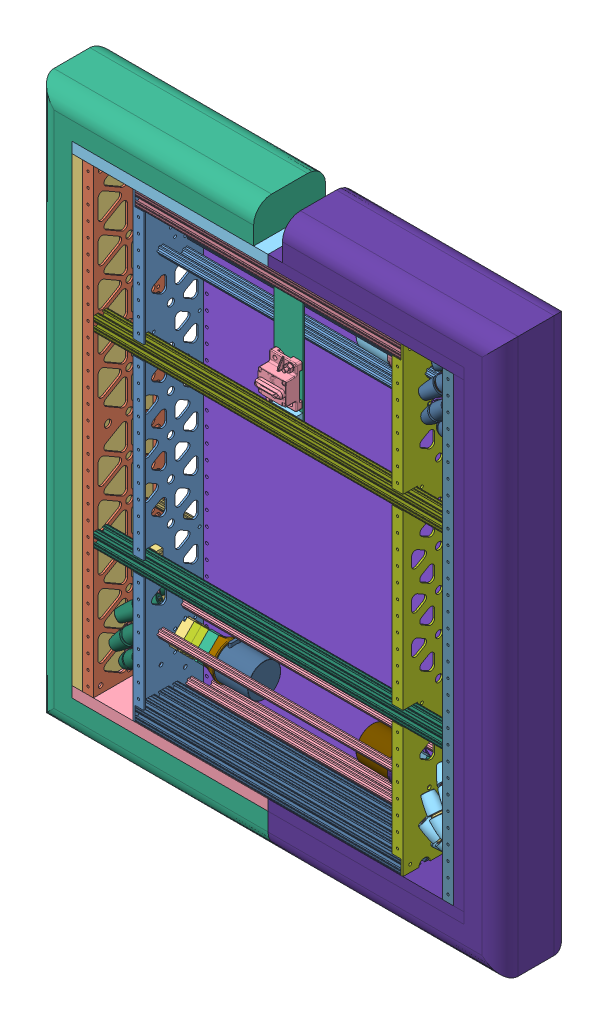
SolidWorks assembly Copy of Fame 2020, configuration Default. Lengths in mm. (continued)
Components (placement in the parent): (continued)
- Left Wheel Assembly v4(Mirror)^Copy of Fame 2020-1: Left Wheel Assembly v4(Mirror)^Copy of Fame 2020 [Default] at (-500 0 0) x (-1 0 0) z (0 0 -1) size (65.82 166.11 165.01) (virtual)
  - 6_Mecanum_Wheel_Left_217-2799 v1(Mirror)^Left Wheel Assembly v4(Mirror)_Copy of Fame 2020-1: 6_Mecanum_Wheel_Left_217-2799 v1(Mirror)^Left Wheel Assembly v4(Mirror)_Copy of Fame 2020 [Default] x (0 0 -1) z (1 0 0) size (165.01 166.11 65.82) (virtual)
    - 217-2799-001 Rev1(Mirror)^6_Mecanum_Wheel_Left_217-2799 v1(Mirror)_Left Wheel Assembly v4(Mirror)_Copy of Fame 2020-1: 217-2799-001 Rev1(Mirror)^6_Mecanum_Wheel_Left_217-2799 v1(Mirror)_Left Wheel Assembly v4(Mirror)_Copy of Fame 2020 [Default] at (33.3875 -317.5 -234.0098) x (0.707107 0.707107 0) z (0 0 1) size (95.78 100.46 28.55) (virtual)
    - 217-2799-001 Rev1(Mirror)^6_Mecanum_Wheel_Left_217-2799 v1(Mirror)_Left Wheel Assembly v4(Mirror)_Copy of Fame 2020-2: 217-2799-001 Rev1(Mirror)^6_Mecanum_Wheel_Left_217-2799 v1(Mirror)_Left Wheel Assembly v4(Mirror)_Copy of Fame 2020 [Default] at (33.3875 -317.5 -221.3098) x (-0.987688 -0.156434 0) z (0 0 -1) size (95.78 100.46 28.55) (virtual)
    - 217-2799-002 Rev1(Mirror)^6_Mecanum_Wheel_Left_217-2799 v1(Mirror)_Left Wheel Assembly v4(Mirror)_Copy of Fame 2020-1: 217-2799-002 Rev1(Mirror)^6_Mecanum_Wheel_Left_217-2799 v1(Mirror)_Left Wheel Assembly v4(Mirror)_Copy of Fame 2020 [Default] at (4.057 -346.8305 -227.6598) x (-0.707107 0.707107 0) z (0.707107 0.707107 0) size (26.84 25.39 30.1) (virtual)
    - 217-2799-002 Rev1(Mirror)^6_Mecanum_Wheel_Left_217-2799 v1(Mirror)_Left Wheel Assembly v4(Mirror)_Copy of Fame 2020-2: 217-2799-002 Rev1(Mirror)^6_Mecanum_Wheel_Left_217-2799 v1(Mirror)_Left Wheel Assembly v4(Mirror)_Copy of Fame 2020 [Default] at (-7.5815 -323.9888 -227.6598) x (-0.156434 0.987688 0) z (0.987688 0.156434 0) size (26.84 25.39 30.1) (virtual)
    - 217-2799-002 Rev1(Mirror)^6_Mecanum_Wheel_Left_217-2799 v1(Mirror)_Left Wheel Assembly v4(Mirror)_Copy of Fame 2020-3: 217-2799-002 Rev1(Mirror)^6_Mecanum_Wheel_Left_217-2799 v1(Mirror)_Left Wheel Assembly v4(Mirror)_Copy of Fame 2020 [Default] at (-3.5711 -298.6686 -227.6598) x (0.45399 0.891007 0) z (0.891007 -0.45399 0) size (26.84 25.39 30.1) (virtual)
    - 217-2799-002 Rev1(Mirror)^6_Mecanum_Wheel_Left_217-2799 v1(Mirror)_Left Wheel Assembly v4(Mirror)_Copy of Fame 2020-4: 217-2799-002 Rev1(Mirror)^6_Mecanum_Wheel_Left_217-2799 v1(Mirror)_Left Wheel Assembly v4(Mirror)_Copy of Fame 2020 [Default] at (14.5561 -280.5414 -227.6598) x (0.891007 0.45399 0) z (0.45399 -0.891007 0) size (26.84 25.39 30.1) (virtual)
    - 217-2799-002 Rev1(Mirror)^6_Mecanum_Wheel_Left_217-2799 v1(Mirror)_Left Wheel Assembly v4(Mirror)_Copy of Fame 2020-5: 217-2799-002 Rev1(Mirror)^6_Mecanum_Wheel_Left_217-2799 v1(Mirror)_Left Wheel Assembly v4(Mirror)_Copy of Fame 2020 [Default] at (39.8763 -276.531 -227.6598) x (0.987688 -0.156434 0) z (-0.156434 -0.987688 0) size (26.84 25.39 30.1) (virtual)
    - 217-2799-002 Rev1(Mirror)^6_Mecanum_Wheel_Left_217-2799 v1(Mirror)_Left Wheel Assembly v4(Mirror)_Copy of Fame 2020-6: 217-2799-002 Rev1(Mirror)^6_Mecanum_Wheel_Left_217-2799 v1(Mirror)_Left Wheel Assembly v4(Mirror)_Copy of Fame 2020 [Default] at (62.718 -288.1695 -227.6598) x (0.707107 -0.707107 0) z (-0.707107 -0.707107 0) size (26.84 25.39 30.1) (virtual)
    - 217-2799-002 Rev1(Mirror)^6_Mecanum_Wheel_Left_217-2799 v1(Mirror)_Left Wheel Assembly v4(Mirror)_Copy of Fame 2020-7: 217-2799-002 Rev1(Mirror)^6_Mecanum_Wheel_Left_217-2799 v1(Mirror)_Left Wheel Assembly v4(Mirror)_Copy of Fame 2020 [Default] at (74.3565 -311.0112 -227.6598) x (0.156434 -0.987688 0) z (-0.987688 -0.156434 0) size (26.84 25.39 30.1) (virtual)
    - 217-2799-002 Rev1(Mirror)^6_Mecanum_Wheel_Left_217-2799 v1(Mirror)_Left Wheel Assembly v4(Mirror)_Copy of Fame 2020-8: 217-2799-002 Rev1(Mirror)^6_Mecanum_Wheel_Left_217-2799 v1(Mirror)_Left Wheel Assembly v4(Mirror)_Copy of Fame 2020 [Default] at (70.3461 -336.3314 -227.6598) x (-0.45399 -0.891007 0) z (-0.891007 0.45399 0) size (26.84 25.39 30.1) (virtual)
    - 217-2799-002 Rev1(Mirror)^6_Mecanum_Wheel_Left_217-2799 v1(Mirror)_Left Wheel Assembly v4(Mirror)_Copy of Fame 2020-9: 217-2799-002 Rev1(Mirror)^6_Mecanum_Wheel_Left_217-2799 v1(Mirror)_Left Wheel Assembly v4(Mirror)_Copy of Fame 2020 [Default] at (52.2189 -354.4586 -227.6598) x (-0.891007 -0.45399 0) z (-0.45399 0.891007 0) size (26.84 25.39 30.1) (virtual)
    - 217-2799-002 Rev1(Mirror)^6_Mecanum_Wheel_Left_217-2799 v1(Mirror)_Left Wheel Assembly v4(Mirror)_Copy of Fame 2020-10: 217-2799-002 Rev1(Mirror)^6_Mecanum_Wheel_Left_217-2799 v1(Mirror)_Left Wheel Assembly v4(Mirror)_Copy of Fame 2020 [Default] at (26.8987 -358.469 -227.6598) x (-0.987688 0.156434 0) z (0.156434 0.987688 0) size (26.84 25.39 30.1) (virtual)
    - 217-2586-003 Rev2(Mirror)^6_Mecanum_Wheel_Left_217-2799 v1(Mirror)_Left Wheel Assembly v4(Mirror)_Copy of Fame 2020-1: 217-2586-003 Rev2(Mirror)^6_Mecanum_Wheel_Left_217-2799 v1(Mirror)_Left Wheel Assembly v4(Mirror)_Copy of Fame 2020 [Default] at (-13.4676 -358.6894 -223.6536) x (0.41944 0.854155 -0.30739) z (0.757674 -0.142894 0.636798) size (19.46 28.57 19.46) (virtual)
    - 217-2586-003 Rev2(Mirror)^6_Mecanum_Wheel_Left_217-2799 v1(Mirror)_Left Wheel Assembly v4(Mirror)_Copy of Fame 2020-2: 217-2586-003 Rev2(Mirror)^6_Mecanum_Wheel_Left_217-2799 v1(Mirror)_Left Wheel Assembly v4(Mirror)_Copy of Fame 2020 [Default] at (-7.8019 -364.3551 -231.666) x (0.847342 0.451134 0.280161) z (-0.17892 0.739241 -0.649238) size (19.46 28.57 19.46) (virtual)
    - 217-2586-003 Rev2(Mirror)^6_Mecanum_Wheel_Left_217-2799 v1(Mirror)_Left Wheel Assembly v4(Mirror)_Copy of Fame 2020-3: 217-2586-003 Rev2(Mirror)^6_Mecanum_Wheel_Left_217-2799 v1(Mirror)_Left Wheel Assembly v4(Mirror)_Copy of Fame 2020 [Default] at (-27.4761 -331.196 -231.666) x (0.950684 -0.13308 0.280161) z (0.289766 0.703225 -0.649238) size (19.46 28.57 19.46) (virtual)
    - 217-2586-003 Rev2(Mirror)^6_Mecanum_Wheel_Left_217-2799 v1(Mirror)_Left Wheel Assembly v4(Mirror)_Copy of Fame 2020-4: 217-2586-003 Rev2(Mirror)^6_Mecanum_Wheel_Left_217-2799 v1(Mirror)_Left Wheel Assembly v4(Mirror)_Copy of Fame 2020 [Default] at (-23.9025 -292.8056 -231.666) x (0.690897 -0.666462 0.280161) z (0.647771 0.398601 -0.649238) size (19.46 28.57 19.46) (virtual)
    - 217-2586-003 Rev2(Mirror)^6_Mecanum_Wheel_Left_217-2799 v1(Mirror)_Left Wheel Assembly v4(Mirror)_Copy of Fame 2020-5: 217-2586-003 Rev2(Mirror)^6_Mecanum_Wheel_Left_217-2799 v1(Mirror)_Left Wheel Assembly v4(Mirror)_Copy of Fame 2020 [Default] at (1.5539 -263.8475 -231.666) x (0.167211 -0.945278 0.280161) z (0.75835 -0.058276 -0.649238) size (19.46 28.57 19.46) (virtual)
    - 217-2586-003 Rev2(Mirror)^6_Mecanum_Wheel_Left_217-2799 v1(Mirror)_Left Wheel Assembly v4(Mirror)_Copy of Fame 2020-6: 217-2586-003 Rev2(Mirror)^6_Mecanum_Wheel_Left_217-2799 v1(Mirror)_Left Wheel Assembly v4(Mirror)_Copy of Fame 2020 [Default] at (39.1697 -255.3829 -231.666) x (-0.420344 -0.86303 0.280161) z (0.579264 -0.492893 -0.649238) size (19.46 28.57 19.46) (virtual)
    - 217-2586-003 Rev2(Mirror)^6_Mecanum_Wheel_Left_217-2799 v1(Mirror)_Left Wheel Assembly v4(Mirror)_Copy of Fame 2020-7: 217-2586-003 Rev2(Mirror)^6_Mecanum_Wheel_Left_217-2799 v1(Mirror)_Left Wheel Assembly v4(Mirror)_Copy of Fame 2020 [Default] at (74.5769 -270.6449 -231.666) x (-0.847342 -0.451134 0.280161) z (0.17892 -0.739241 -0.649238) size (19.46 28.57 19.46) (virtual)
    - 217-2586-003 Rev2(Mirror)^6_Mecanum_Wheel_Left_217-2799 v1(Mirror)_Left Wheel Assembly v4(Mirror)_Copy of Fame 2020-8: 217-2586-003 Rev2(Mirror)^6_Mecanum_Wheel_Left_217-2799 v1(Mirror)_Left Wheel Assembly v4(Mirror)_Copy of Fame 2020 [Default] at (94.2511 -303.804 -231.666) x (-0.950684 0.13308 0.280161) z (-0.289766 -0.703225 -0.649238) size (19.46 28.57 19.46) (virtual)
    - 217-2586-003 Rev2(Mirror)^6_Mecanum_Wheel_Left_217-2799 v1(Mirror)_Left Wheel Assembly v4(Mirror)_Copy of Fame 2020-9: 217-2586-003 Rev2(Mirror)^6_Mecanum_Wheel_Left_217-2799 v1(Mirror)_Left Wheel Assembly v4(Mirror)_Copy of Fame 2020 [Default] at (90.6775 -342.1944 -231.666) x (-0.690897 0.666462 0.280161) z (-0.647771 -0.398601 -0.649238) size (19.46 28.57 19.46) (virtual)
    - 217-2586-003 Rev2(Mirror)^6_Mecanum_Wheel_Left_217-2799 v1(Mirror)_Left Wheel Assembly v4(Mirror)_Copy of Fame 2020-10: 217-2586-003 Rev2(Mirror)^6_Mecanum_Wheel_Left_217-2799 v1(Mirror)_Left Wheel Assembly v4(Mirror)_Copy of Fame 2020 [Default] at (65.2211 -371.1525 -231.666) x (-0.167211 0.945278 0.280161) z (-0.75835 0.058276 -0.649238) size (19.46 28.57 19.46) (virtual)
    - 217-2586-003 Rev2(Mirror)^6_Mecanum_Wheel_Left_217-2799 v1(Mirror)_Left Wheel Assembly v4(Mirror)_Copy of Fame 2020-11: 217-2586-003 Rev2(Mirror)^6_Mecanum_Wheel_Left_217-2799 v1(Mirror)_Left Wheel Assembly v4(Mirror)_Copy of Fame 2020 [Default] at (27.6053 -379.6171 -231.666) x (0.420344 0.86303 0.280161) z (-0.579264 0.492893 -0.649238) size (19.46 28.57 19.46) (virtual)
    - 217-2586-003 Rev2(Mirror)^6_Mecanum_Wheel_Left_217-2799 v1(Mirror)_Left Wheel Assembly v4(Mirror)_Copy of Fame 2020-12: 217-2586-003 Rev2(Mirror)^6_Mecanum_Wheel_Left_217-2799 v1(Mirror)_Left Wheel Assembly v4(Mirror)_Copy of Fame 2020 [Default] at (-28.7296 -323.2822 -223.6536) x (0.841394 0.444485 -0.30739) z (0.52898 -0.560953 0.636798) size (19.46 28.57 19.46) (virtual)
    - 217-2586-003 Rev2(Mirror)^6_Mecanum_Wheel_Left_217-2799 v1(Mirror)_Left Wheel Assembly v4(Mirror)_Copy of Fame 2020-13: 217-2586-003 Rev2(Mirror)^6_Mecanum_Wheel_Left_217-2799 v1(Mirror)_Left Wheel Assembly v4(Mirror)_Copy of Fame 2020 [Default] at (-20.265 -285.6664 -223.6536) x (0.941964 -0.134963 -0.30739) z (0.098234 -0.764747 0.636798) size (19.46 28.57 19.46) (virtual)
    - 217-2586-003 Rev2(Mirror)^6_Mecanum_Wheel_Left_217-2799 v1(Mirror)_Left Wheel Assembly v4(Mirror)_Copy of Fame 2020-14: 217-2586-003 Rev2(Mirror)^6_Mecanum_Wheel_Left_217-2799 v1(Mirror)_Left Wheel Assembly v4(Mirror)_Copy of Fame 2020 [Default] at (8.6931 -260.21 -223.6536) x (0.682736 -0.66286 -0.30739) z (-0.370035 -0.676434 0.636798) size (19.46 28.57 19.46) (virtual)
    - 217-2586-003 Rev2(Mirror)^6_Mecanum_Wheel_Left_217-2799 v1(Mirror)_Left Wheel Assembly v4(Mirror)_Copy of Fame 2020-15: 217-2586-003 Rev2(Mirror)^6_Mecanum_Wheel_Left_217-2799 v1(Mirror)_Left Wheel Assembly v4(Mirror)_Copy of Fame 2020 [Default] at (47.0835 -256.6364 -223.6536) x (0.162726 -0.937567 -0.30739) z (-0.696962 -0.329746 0.636798) size (19.46 28.57 19.46) (virtual)
    - 217-2586-003 Rev2(Mirror)^6_Mecanum_Wheel_Left_217-2799 v1(Mirror)_Left Wheel Assembly v4(Mirror)_Copy of Fame 2020-16: 217-2586-003 Rev2(Mirror)^6_Mecanum_Wheel_Left_217-2799 v1(Mirror)_Left Wheel Assembly v4(Mirror)_Copy of Fame 2020 [Default] at (80.2426 -276.3106 -223.6536) x (-0.41944 -0.854155 -0.30739) z (-0.757674 0.142894 0.636798) size (19.46 28.57 19.46) (virtual)
    - 217-2586-003 Rev2(Mirror)^6_Mecanum_Wheel_Left_217-2799 v1(Mirror)_Left Wheel Assembly v4(Mirror)_Copy of Fame 2020-17: 217-2586-003 Rev2(Mirror)^6_Mecanum_Wheel_Left_217-2799 v1(Mirror)_Left Wheel Assembly v4(Mirror)_Copy of Fame 2020 [Default] at (95.5046 -311.7178 -223.6536) x (-0.841394 -0.444485 -0.30739) z (-0.52898 0.560953 0.636798) size (19.46 28.57 19.46) (virtual)
    - 217-2586-003 Rev2(Mirror)^6_Mecanum_Wheel_Left_217-2799 v1(Mirror)_Left Wheel Assembly v4(Mirror)_Copy of Fame 2020-18: 217-2586-003 Rev2(Mirror)^6_Mecanum_Wheel_Left_217-2799 v1(Mirror)_Left Wheel Assembly v4(Mirror)_Copy of Fame 2020 [Default] at (87.04 -349.3336 -223.6536) x (-0.941964 0.134963 -0.30739) z (-0.098234 0.764747 0.636798) size (19.46 28.57 19.46) (virtual)
    - 217-2586-003 Rev2(Mirror)^6_Mecanum_Wheel_Left_217-2799 v1(Mirror)_Left Wheel Assembly v4(Mirror)_Copy of Fame 2020-19: 217-2586-003 Rev2(Mirror)^6_Mecanum_Wheel_Left_217-2799 v1(Mirror)_Left Wheel Assembly v4(Mirror)_Copy of Fame 2020 [Default] at (58.0819 -374.79 -223.6536) x (-0.682736 0.66286 -0.30739) z (0.370035 0.676434 0.636798) size (19.46 28.57 19.46) (virtual)
    - 217-2586-003 Rev2(Mirror)^6_Mecanum_Wheel_Left_217-2799 v1(Mirror)_Left Wheel Assembly v4(Mirror)_Copy of Fame 2020-20: 217-2586-003 Rev2(Mirror)^6_Mecanum_Wheel_Left_217-2799 v1(Mirror)_Left Wheel Assembly v4(Mirror)_Copy of Fame 2020 [Default] at (19.6915 -378.3636 -223.6536) x (-0.162726 0.937567 -0.30739) z (0.696962 0.329746 0.636798) size (19.46 28.57 19.46) (virtual)
    - 217-2586-004 Rev1(Mirror)^6_Mecanum_Wheel_Left_217-2799 v1(Mirror)_Left Wheel Assembly v4(Mirror)_Copy of Fame 2020-1: 217-2586-004 Rev1(Mirror)^6_Mecanum_Wheel_Left_217-2799 v1(Mirror)_Left Wheel Assembly v4(Mirror)_Copy of Fame 2020 [Default] at (-10.3479 -361.809 -228.0654) x (-0.690521 -0.722949 0.02293) z (-0.522667 0.476807 -0.706735) size (25.9 28.58 25.9) (virtual)
    - 217-2586-004 Rev1(Mirror)^6_Mecanum_Wheel_Left_217-2799 v1(Mirror)_Left Wheel Assembly v4(Mirror)_Copy of Fame 2020-2: 217-2586-004 Rev1(Mirror)^6_Mecanum_Wheel_Left_217-2799 v1(Mirror)_Left Wheel Assembly v4(Mirror)_Copy of Fame 2020 [Default] at (-10.9209 -361.2361 -227.2551) x (0.01458 -0.811521 0.584142) z (0.865903 0.302381 0.39847) size (25.9 28.58 25.9) (virtual)
    - 217-2586-004 Rev1(Mirror)^6_Mecanum_Wheel_Left_217-2799 v1(Mirror)_Left Wheel Assembly v4(Mirror)_Copy of Fame 2020-3: 217-2586-004 Rev1(Mirror)^6_Mecanum_Wheel_Left_217-2799 v1(Mirror)_Left Wheel Assembly v4(Mirror)_Copy of Fame 2020 [Default] at (-28.1662 -326.8394 -227.2551) x (-0.465204 -0.665104 0.584142) z (0.878265 -0.264334 0.39847) size (25.9 28.58 25.9) (virtual)
    - 217-2586-004 Rev1(Mirror)^6_Mecanum_Wheel_Left_217-2799 v1(Mirror)_Left Wheel Assembly v4(Mirror)_Copy of Fame 2020-4: 217-2586-004 Rev1(Mirror)^6_Mecanum_Wheel_Left_217-2799 v1(Mirror)_Left Wheel Assembly v4(Mirror)_Copy of Fame 2020 [Default] at (-21.9 -288.8754 -227.2551) x (-0.767297 -0.26464 0.584142) z (0.55516 -0.730082 0.39847) size (25.9 28.58 25.9) (virtual)
    - 217-2586-004 Rev1(Mirror)^6_Mecanum_Wheel_Left_217-2799 v1(Mirror)_Left Wheel Assembly v4(Mirror)_Copy of Fame 2020-5: 217-2586-004 Rev1(Mirror)^6_Mecanum_Wheel_Left_217-2799 v1(Mirror)_Left Wheel Assembly v4(Mirror)_Copy of Fame 2020 [Default] at (5.484 -261.845 -227.2551) x (-0.776308 0.236907 0.584142) z (0.020002 -0.916963 0.39847) size (25.9 28.58 25.9) (virtual)
    - 217-2586-004 Rev1(Mirror)^6_Mecanum_Wheel_Left_217-2799 v1(Mirror)_Left Wheel Assembly v4(Mirror)_Copy of Fame 2020-6: 217-2586-004 Rev1(Mirror)^6_Mecanum_Wheel_Left_217-2799 v1(Mirror)_Left Wheel Assembly v4(Mirror)_Copy of Fame 2020 [Default] at (43.5263 -256.0729 -227.2551) x (-0.488796 0.647964 0.584142) z (-0.522795 -0.753596 0.39847) size (25.9 28.58 25.9) (virtual)
    - 217-2586-004 Rev1(Mirror)^6_Mecanum_Wheel_Left_217-2799 v1(Mirror)_Left Wheel Assembly v4(Mirror)_Copy of Fame 2020-7: 217-2586-004 Rev1(Mirror)^6_Mecanum_Wheel_Left_217-2799 v1(Mirror)_Left Wheel Assembly v4(Mirror)_Copy of Fame 2020 [Default] at (77.6959 -273.7639 -227.2551) x (-0.01458 0.811521 0.584142) z (-0.865903 -0.302381 0.39847) size (25.9 28.58 25.9) (virtual)
    - 217-2586-004 Rev1(Mirror)^6_Mecanum_Wheel_Left_217-2799 v1(Mirror)_Left Wheel Assembly v4(Mirror)_Copy of Fame 2020-8: 217-2586-004 Rev1(Mirror)^6_Mecanum_Wheel_Left_217-2799 v1(Mirror)_Left Wheel Assembly v4(Mirror)_Copy of Fame 2020 [Default] at (94.9412 -308.1606 -227.2551) x (0.465204 0.665104 0.584142) z (-0.878265 0.264334 0.39847) size (25.9 28.58 25.9) (virtual)
    - 217-2586-004 Rev1(Mirror)^6_Mecanum_Wheel_Left_217-2799 v1(Mirror)_Left Wheel Assembly v4(Mirror)_Copy of Fame 2020-9: 217-2586-004 Rev1(Mirror)^6_Mecanum_Wheel_Left_217-2799 v1(Mirror)_Left Wheel Assembly v4(Mirror)_Copy of Fame 2020 [Default] at (88.675 -346.1246 -227.2551) x (0.767297 0.26464 0.584142) z (-0.55516 0.730082 0.39847) size (25.9 28.58 25.9) (virtual)
    - 217-2586-004 Rev1(Mirror)^6_Mecanum_Wheel_Left_217-2799 v1(Mirror)_Left Wheel Assembly v4(Mirror)_Copy of Fame 2020-10: 217-2586-004 Rev1(Mirror)^6_Mecanum_Wheel_Left_217-2799 v1(Mirror)_Left Wheel Assembly v4(Mirror)_Copy of Fame 2020 [Default] at (61.291 -373.155 -227.2551) x (0.776308 -0.236907 0.584142) z (-0.020002 0.916963 0.39847) size (25.9 28.58 25.9) (virtual)
    - 217-2586-004 Rev1(Mirror)^6_Mecanum_Wheel_Left_217-2799 v1(Mirror)_Left Wheel Assembly v4(Mirror)_Copy of Fame 2020-11: 217-2586-004 Rev1(Mirror)^6_Mecanum_Wheel_Left_217-2799 v1(Mirror)_Left Wheel Assembly v4(Mirror)_Copy of Fame 2020 [Default] at (23.2487 -378.9271 -227.2551) x (0.488796 -0.647964 0.584142) z (0.522795 0.753596 0.39847) size (25.9 28.58 25.9) (virtual)
    - 217-2586-004 Rev1(Mirror)^6_Mecanum_Wheel_Left_217-2799 v1(Mirror)_Left Wheel Assembly v4(Mirror)_Copy of Fame 2020-12: 217-2586-004 Rev1(Mirror)^6_Mecanum_Wheel_Left_217-2799 v1(Mirror)_Left Wheel Assembly v4(Mirror)_Copy of Fame 2020 [Default] at (-28.0394 -327.6397 -228.0654) x (-0.983582 -0.179 0.02293) z (-0.142587 0.692961 -0.706735) size (25.9 28.58 25.9) (virtual)
    - 217-2586-004 Rev1(Mirror)^6_Mecanum_Wheel_Left_217-2799 v1(Mirror)_Left Wheel Assembly v4(Mirror)_Copy of Fame 2020-13: 217-2586-004 Rev1(Mirror)^6_Mecanum_Wheel_Left_217-2799 v1(Mirror)_Left Wheel Assembly v4(Mirror)_Copy of Fame 2020 [Default] at (-22.2679 -289.5974 -228.0654) x (-0.900948 0.433321 0.02293) z (0.291957 0.644427 -0.706735) size (25.9 28.58 25.9) (virtual)
    - 217-2586-004 Rev1(Mirror)^6_Mecanum_Wheel_Left_217-2799 v1(Mirror)_Left Wheel Assembly v4(Mirror)_Copy of Fame 2020-14: 217-2586-004 Rev1(Mirror)^6_Mecanum_Wheel_Left_217-2799 v1(Mirror)_Left Wheel Assembly v4(Mirror)_Copy of Fame 2020 [Default] at (4.7621 -262.2129 -228.0654) x (-0.474183 0.880128 0.02293) z (0.614983 0.349745 -0.706735) size (25.9 28.58 25.9) (virtual)
    - 217-2586-004 Rev1(Mirror)^6_Mecanum_Wheel_Left_217-2799 v1(Mirror)_Left Wheel Assembly v4(Mirror)_Copy of Fame 2020-15: 217-2586-004 Rev1(Mirror)^6_Mecanum_Wheel_Left_217-2799 v1(Mirror)_Left Wheel Assembly v4(Mirror)_Copy of Fame 2020 [Default] at (42.726 -255.9462 -228.0654) x (0.133704 0.990756 0.02293) z (0.703107 -0.078529 -0.706735) size (25.9 28.58 25.9) (virtual)
    - 217-2586-004 Rev1(Mirror)^6_Mecanum_Wheel_Left_217-2799 v1(Mirror)_Left Wheel Assembly v4(Mirror)_Copy of Fame 2020-16: 217-2586-004 Rev1(Mirror)^6_Mecanum_Wheel_Left_217-2799 v1(Mirror)_Left Wheel Assembly v4(Mirror)_Copy of Fame 2020 [Default] at (77.1229 -273.191 -228.0654) x (0.690521 0.722949 0.02293) z (0.522667 -0.476807 -0.706735) size (25.9 28.58 25.9) (virtual)
    - 217-2586-004 Rev1(Mirror)^6_Mecanum_Wheel_Left_217-2799 v1(Mirror)_Left Wheel Assembly v4(Mirror)_Copy of Fame 2020-17: 217-2586-004 Rev1(Mirror)^6_Mecanum_Wheel_Left_217-2799 v1(Mirror)_Left Wheel Assembly v4(Mirror)_Copy of Fame 2020 [Default] at (94.8144 -307.3603 -228.0654) x (0.983582 0.179 0.02293) z (0.142587 -0.692961 -0.706735) size (25.9 28.58 25.9) (virtual)
    - 217-2586-004 Rev1(Mirror)^6_Mecanum_Wheel_Left_217-2799 v1(Mirror)_Left Wheel Assembly v4(Mirror)_Copy of Fame 2020-18: 217-2586-004 Rev1(Mirror)^6_Mecanum_Wheel_Left_217-2799 v1(Mirror)_Left Wheel Assembly v4(Mirror)_Copy of Fame 2020 [Default] at (89.0429 -345.4026 -228.0654) x (0.900948 -0.433321 0.02293) z (-0.291957 -0.644427 -0.706735) size (25.9 28.58 25.9) (virtual)
    - 217-2586-004 Rev1(Mirror)^6_Mecanum_Wheel_Left_217-2799 v1(Mirror)_Left Wheel Assembly v4(Mirror)_Copy of Fame 2020-19: 217-2586-004 Rev1(Mirror)^6_Mecanum_Wheel_Left_217-2799 v1(Mirror)_Left Wheel Assembly v4(Mirror)_Copy of Fame 2020 [Default] at (62.0129 -372.7871 -228.0654) x (0.474183 -0.880128 0.02293) z (-0.614983 -0.349745 -0.706735) size (25.9 28.58 25.9) (virtual)
    - 217-2586-004 Rev1(Mirror)^6_Mecanum_Wheel_Left_217-2799 v1(Mirror)_Left Wheel Assembly v4(Mirror)_Copy of Fame 2020-20: 217-2586-004 Rev1(Mirror)^6_Mecanum_Wheel_Left_217-2799 v1(Mirror)_Left Wheel Assembly v4(Mirror)_Copy of Fame 2020 [Default] at (24.049 -379.0538 -228.0654) x (-0.133704 -0.990756 0.02293) z (-0.703107 0.078529 -0.706735) size (25.9 28.58 25.9) (virtual)
    - 217-2586-007 Rev1(Mirror)^6_Mecanum_Wheel_Left_217-2799 v1(Mirror)_Left Wheel Assembly v4(Mirror)_Copy of Fame 2020-1: 217-2586-007 Rev1(Mirror)^6_Mecanum_Wheel_Left_217-2799 v1(Mirror)_Left Wheel Assembly v4(Mirror)_Copy of Fame 2020 [Default] at (-10.6347 -361.5222 -227.6598) x (0.5 -0.5 -0.707107) z (0.709055 0.705148 0.002763) size (61.72 5 5) (virtual)
    - 217-2586-007 Rev1(Mirror)^6_Mecanum_Wheel_Left_217-2799 v1(Mirror)_Left Wheel Assembly v4(Mirror)_Copy of Fame 2020-2: 217-2586-007 Rev1(Mirror)^6_Mecanum_Wheel_Left_217-2799 v1(Mirror)_Left Wheel Assembly v4(Mirror)_Copy of Fame 2020 [Default] at (-28.1029 -327.2391 -227.6598) x (0.110616 -0.698401 -0.707107) z (0.988113 0.153705 0.002763) size (61.72 5 5) (virtual)
    - 217-2586-007 Rev1(Mirror)^6_Mecanum_Wheel_Left_217-2799 v1(Mirror)_Left Wheel Assembly v4(Mirror)_Copy of Fame 2020-3: 217-2586-007 Rev1(Mirror)^6_Mecanum_Wheel_Left_217-2799 v1(Mirror)_Left Wheel Assembly v4(Mirror)_Copy of Fame 2020 [Default] at (-22.0838 -289.236 -227.6598) x (-0.32102 -0.630037 -0.707107) z (0.889746 -0.456448 0.002763) size (61.72 5 5) (virtual)
    - 217-2586-007 Rev1(Mirror)^6_Mecanum_Wheel_Left_217-2799 v1(Mirror)_Left Wheel Assembly v4(Mirror)_Copy of Fame 2020-4: 217-2586-007 Rev1(Mirror)^6_Mecanum_Wheel_Left_217-2799 v1(Mirror)_Left Wheel Assembly v4(Mirror)_Copy of Fame 2020 [Default] at (5.1235 -262.0287 -227.6598) x (-0.630037 -0.32102 -0.707107) z (0.451526 -0.892254 0.002763) size (61.72 5 5) (virtual)
    - 217-2586-007 Rev1(Mirror)^6_Mecanum_Wheel_Left_217-2799 v1(Mirror)_Left Wheel Assembly v4(Mirror)_Copy of Fame 2020-5: 217-2586-007 Rev1(Mirror)^6_Mecanum_Wheel_Left_217-2799 v1(Mirror)_Left Wheel Assembly v4(Mirror)_Copy of Fame 2020 [Default] at (43.1266 -256.0096 -227.6598) x (-0.698401 0.110616 -0.707107) z (-0.159162 -0.987249 0.002763) size (61.72 5 5) (virtual)
    - 217-2586-007 Rev1(Mirror)^6_Mecanum_Wheel_Left_217-2799 v1(Mirror)_Left Wheel Assembly v4(Mirror)_Copy of Fame 2020-6: 217-2586-007 Rev1(Mirror)^6_Mecanum_Wheel_Left_217-2799 v1(Mirror)_Left Wheel Assembly v4(Mirror)_Copy of Fame 2020 [Default] at (77.4097 -273.4778 -227.6598) x (-0.5 0.5 -0.707107) z (-0.709055 -0.705148 0.002763) size (61.72 5 5) (virtual)
    - 217-2586-007 Rev1(Mirror)^6_Mecanum_Wheel_Left_217-2799 v1(Mirror)_Left Wheel Assembly v4(Mirror)_Copy of Fame 2020-7: 217-2586-007 Rev1(Mirror)^6_Mecanum_Wheel_Left_217-2799 v1(Mirror)_Left Wheel Assembly v4(Mirror)_Copy of Fame 2020 [Default] at (94.8779 -307.7609 -227.6598) x (-0.110616 0.698401 -0.707107) z (-0.988113 -0.153705 0.002763) size (61.72 5 5) (virtual)
    - 217-2586-007 Rev1(Mirror)^6_Mecanum_Wheel_Left_217-2799 v1(Mirror)_Left Wheel Assembly v4(Mirror)_Copy of Fame 2020-8: 217-2586-007 Rev1(Mirror)^6_Mecanum_Wheel_Left_217-2799 v1(Mirror)_Left Wheel Assembly v4(Mirror)_Copy of Fame 2020 [Default] at (88.8588 -345.764 -227.6598) x (0.32102 0.630037 -0.707107) z (-0.889746 0.456448 0.002763) size (61.72 5 5) (virtual)
    - 217-2586-007 Rev1(Mirror)^6_Mecanum_Wheel_Left_217-2799 v1(Mirror)_Left Wheel Assembly v4(Mirror)_Copy of Fame 2020-9: 217-2586-007 Rev1(Mirror)^6_Mecanum_Wheel_Left_217-2799 v1(Mirror)_Left Wheel Assembly v4(Mirror)_Copy of Fame 2020 [Default] at (61.6515 -372.9713 -227.6598) x (0.630037 0.32102 -0.707107) z (-0.451526 0.892254 0.002763) size (61.72 5 5) (virtual)
    - 217-2586-007 Rev1(Mirror)^6_Mecanum_Wheel_Left_217-2799 v1(Mirror)_Left Wheel Assembly v4(Mirror)_Copy of Fame 2020-10: 217-2586-007 Rev1(Mirror)^6_Mecanum_Wheel_Left_217-2799 v1(Mirror)_Left Wheel Assembly v4(Mirror)_Copy of Fame 2020 [Default] at (23.6484 -378.9904 -227.6598) x (0.698401 -0.110616 -0.707107) z (0.159162 0.987249 0.002763) size (61.72 5 5) (virtual)
    - 217-2586-008 Rev1(Mirror)^6_Mecanum_Wheel_Left_217-2799 v1(Mirror)_Left Wheel Assembly v4(Mirror)_Copy of Fame 2020-1: 217-2586-008 Rev1(Mirror)^6_Mecanum_Wheel_Left_217-2799 v1(Mirror)_Left Wheel Assembly v4(Mirror)_Copy of Fame 2020 [Default] at (53.3583 -330.4692 -227.5328) x (0.544639 0.838671 0) z (0 0 -1) size (7.33 6.35 31.75) (virtual)
    - 217-2586-008 Rev1(Mirror)^6_Mecanum_Wheel_Left_217-2799 v1(Mirror)_Left Wheel Assembly v4(Mirror)_Copy of Fame 2020-2: 217-2586-008 Rev1(Mirror)^6_Mecanum_Wheel_Left_217-2799 v1(Mirror)_Left Wheel Assembly v4(Mirror)_Copy of Fame 2020 [Default] at (32.1413 -341.2799 -227.5328) x (0.99863 -0.052336 0) z (0 0 -1) size (7.33 6.35 31.75) (virtual)
    - 217-2586-008 Rev1(Mirror)^6_Mecanum_Wheel_Left_217-2799 v1(Mirror)_Left Wheel Assembly v4(Mirror)_Copy of Fame 2020-3: 217-2586-008 Rev1(Mirror)^6_Mecanum_Wheel_Left_217-2799 v1(Mirror)_Left Wheel Assembly v4(Mirror)_Copy of Fame 2020 [Default] at (12.1704 -328.3106 -227.5328) x (0.45399 -0.891007 0) z (0 0 -1) size (7.33 6.35 31.75) (virtual)
    - 217-2586-008 Rev1(Mirror)^6_Mecanum_Wheel_Left_217-2799 v1(Mirror)_Left Wheel Assembly v4(Mirror)_Copy of Fame 2020-4: 217-2586-008 Rev1(Mirror)^6_Mecanum_Wheel_Left_217-2799 v1(Mirror)_Left Wheel Assembly v4(Mirror)_Copy of Fame 2020 [Default] at (13.4167 -304.5308 -227.5328) x (-0.544639 -0.838671 0) z (0 0 -1) size (7.33 6.35 31.75) (virtual)
    - 217-2586-008 Rev1(Mirror)^6_Mecanum_Wheel_Left_217-2799 v1(Mirror)_Left Wheel Assembly v4(Mirror)_Copy of Fame 2020-5: 217-2586-008 Rev1(Mirror)^6_Mecanum_Wheel_Left_217-2799 v1(Mirror)_Left Wheel Assembly v4(Mirror)_Copy of Fame 2020 [Default] at (34.6337 -293.7201 -227.5328) x (-0.99863 0.052336 0) z (0 0 -1) size (7.33 6.35 31.75) (virtual)
    - 217-2586-008 Rev1(Mirror)^6_Mecanum_Wheel_Left_217-2799 v1(Mirror)_Left Wheel Assembly v4(Mirror)_Copy of Fame 2020-6: 217-2586-008 Rev1(Mirror)^6_Mecanum_Wheel_Left_217-2799 v1(Mirror)_Left Wheel Assembly v4(Mirror)_Copy of Fame 2020 [Default] at (54.6046 -306.6894 -227.5328) x (-0.45399 0.891007 0) z (0 0 -1) size (7.33 6.35 31.75) (virtual)
    - NUT-832-NYLOCK(Mirror)^6_Mecanum_Wheel_Left_217-2799 v1(Mirror)_Left Wheel Assembly v4(Mirror)_Copy of Fame 2020-1: NUT-832-NYLOCK(Mirror)^6_Mecanum_Wheel_Left_217-2799 v1(Mirror)_Left Wheel Assembly v4(Mirror)_Copy of Fame 2020 [Default] at (6.1639 -290.2764 -241.3161) x (0.258819 -0.965926 0) z (0.965926 0.258819 0) size (9.37 5.86 8.12) (virtual)
    - NUT-832-NYLOCK(Mirror)^6_Mecanum_Wheel_Left_217-2799 v1(Mirror)_Left Wheel Assembly v4(Mirror)_Copy of Fame 2020-2: NUT-832-NYLOCK(Mirror)^6_Mecanum_Wheel_Left_217-2799 v1(Mirror)_Left Wheel Assembly v4(Mirror)_Copy of Fame 2020 [Default] at (-0.9163 -334.9786 -241.3161) x (0.99863 -0.052336 0) z (0.052336 0.99863 0) size (9.37 5.86 8.12) (virtual)
    - NUT-832-NYLOCK(Mirror)^6_Mecanum_Wheel_Left_217-2799 v1(Mirror)_Left Wheel Assembly v4(Mirror)_Copy of Fame 2020-3: NUT-832-NYLOCK(Mirror)^6_Mecanum_Wheel_Left_217-2799 v1(Mirror)_Left Wheel Assembly v4(Mirror)_Copy of Fame 2020 [Default] at (39.4102 -355.526 -241.3161) x (0.358368 0.93358 0) z (-0.93358 0.358368 0) size (9.37 5.86 8.12) (virtual)
    - NUT-832-NYLOCK(Mirror)^6_Mecanum_Wheel_Left_217-2799 v1(Mirror)_Left Wheel Assembly v4(Mirror)_Copy of Fame 2020-4: NUT-832-NYLOCK(Mirror)^6_Mecanum_Wheel_Left_217-2799 v1(Mirror)_Left Wheel Assembly v4(Mirror)_Copy of Fame 2020 [Default] at (71.4135 -323.5227 -241.3161) x (-0.777146 0.62932 0) z (-0.62932 -0.777146 0) size (9.37 5.86 8.12) (virtual)
    - NUT-832-NYLOCK(Mirror)^6_Mecanum_Wheel_Left_217-2799 v1(Mirror)_Left Wheel Assembly v4(Mirror)_Copy of Fame 2020-5: NUT-832-NYLOCK(Mirror)^6_Mecanum_Wheel_Left_217-2799 v1(Mirror)_Left Wheel Assembly v4(Mirror)_Copy of Fame 2020 [Default] at (50.8661 -283.1962 -241.3161) x (-0.838671 -0.544639 0) z (0.544639 -0.838671 0) size (9.37 5.86 8.12) (virtual)
    - SCREW-832-1250(Mirror)^6_Mecanum_Wheel_Left_217-2799 v1(Mirror)_Left Wheel Assembly v4(Mirror)_Copy of Fame 2020-1: SCREW-832-1250(Mirror)^6_Mecanum_Wheel_Left_217-2799 v1(Mirror)_Left Wheel Assembly v4(Mirror)_Copy of Fame 2020 [Default] at (6.1639 -290.2764 -212.75) x (0 0 -1) z (0.394243 -0.919006 0) size (33.96 7.92 7.92) (virtual)
    - SCREW-832-1250(Mirror)^6_Mecanum_Wheel_Left_217-2799 v1(Mirror)_Left Wheel Assembly v4(Mirror)_Copy of Fame 2020-2: SCREW-832-1250(Mirror)^6_Mecanum_Wheel_Left_217-2799 v1(Mirror)_Left Wheel Assembly v4(Mirror)_Copy of Fame 2020 [Default] at (-0.9163 -334.9786 -212.75) x (0 0 -1) z (0.995855 0.090959 0) size (33.96 7.92 7.92) (virtual)
    - SCREW-832-1250(Mirror)^6_Mecanum_Wheel_Left_217-2799 v1(Mirror)_Left Wheel Assembly v4(Mirror)_Copy of Fame 2020-3: SCREW-832-1250(Mirror)^6_Mecanum_Wheel_Left_217-2799 v1(Mirror)_Left Wheel Assembly v4(Mirror)_Copy of Fame 2020 [Default] at (39.4102 -355.526 -212.75) x (0 0 -1) z (0.221229 0.975222 0) size (33.96 7.92 7.92) (virtual)
    - SCREW-832-1250(Mirror)^6_Mecanum_Wheel_Left_217-2799 v1(Mirror)_Left Wheel Assembly v4(Mirror)_Copy of Fame 2020-4: SCREW-832-1250(Mirror)^6_Mecanum_Wheel_Left_217-2799 v1(Mirror)_Left Wheel Assembly v4(Mirror)_Copy of Fame 2020 [Default] at (71.4135 -323.5227 -212.75) x (0 0 -1) z (-0.859128 0.511761 0) size (33.96 7.92 7.92) (virtual)
    - SCREW-832-1250(Mirror)^6_Mecanum_Wheel_Left_217-2799 v1(Mirror)_Left Wheel Assembly v4(Mirror)_Copy of Fame 2020-5: SCREW-832-1250(Mirror)^6_Mecanum_Wheel_Left_217-2799 v1(Mirror)_Left Wheel Assembly v4(Mirror)_Copy of Fame 2020 [Default] at (50.8661 -283.1962 -212.75) x (0 0 -1) z (-0.752199 -0.658936 0) size (33.96 7.92 7.92) (virtual)
    - 217-2586-005 Rev2(Mirror)^6_Mecanum_Wheel_Left_217-2799 v1(Mirror)_Left Wheel Assembly v4(Mirror)_Copy of Fame 2020-1: 217-2586-005 Rev2(Mirror)^6_Mecanum_Wheel_Left_217-2799 v1(Mirror)_Left Wheel Assembly v4(Mirror)_Copy of Fame 2020 [Default] at (-6.1597 -365.9972 -233.9884) x (-0.5 0.5 0.707107) z (-0.146447 -0.853553 0.5) size (8.5 8 8) (virtual)
    - 217-2586-005 Rev2(Mirror)^6_Mecanum_Wheel_Left_217-2799 v1(Mirror)_Left Wheel Assembly v4(Mirror)_Copy of Fame 2020-2: 217-2586-005 Rev2(Mirror)^6_Mecanum_Wheel_Left_217-2799 v1(Mirror)_Left Wheel Assembly v4(Mirror)_Copy of Fame 2020 [Default] at (-15.1097 -357.0472 -221.3312) x (-0.5 0.5 0.707107) z (-0.146447 -0.853553 0.5) size (8.5 8 8) (virtual)
    - 217-2586-005 Rev2(Mirror)^6_Mecanum_Wheel_Left_217-2799 v1(Mirror)_Left Wheel Assembly v4(Mirror)_Copy of Fame 2020-3: 217-2586-005 Rev2(Mirror)^6_Mecanum_Wheel_Left_217-2799 v1(Mirror)_Left Wheel Assembly v4(Mirror)_Copy of Fame 2020 [Default] at (-29.0929 -320.9884 -221.3312) x (-0.110616 0.698401 0.707107) z (-0.620184 -0.60446 0.5) size (8.5 8 8) (virtual)
    - 217-2586-005 Rev2(Mirror)^6_Mecanum_Wheel_Left_217-2799 v1(Mirror)_Left Wheel Assembly v4(Mirror)_Copy of Fame 2020-4: 217-2586-005 Rev2(Mirror)^6_Mecanum_Wheel_Left_217-2799 v1(Mirror)_Left Wheel Assembly v4(Mirror)_Copy of Fame 2020 [Default] at (-19.2106 -283.5972 -221.3312) x (0.32102 0.630037 0.707107) z (-0.857032 -0.124484 0.5) size (8.5 8 8) (virtual)
    - 217-2586-005 Rev2(Mirror)^6_Mecanum_Wheel_Left_217-2799 v1(Mirror)_Left Wheel Assembly v4(Mirror)_Copy of Fame 2020-5: 217-2586-005 Rev2(Mirror)^6_Mecanum_Wheel_Left_217-2799 v1(Mirror)_Left Wheel Assembly v4(Mirror)_Copy of Fame 2020 [Default] at (10.7623 -259.1556 -221.3312) x (0.630037 0.32102 0.707107) z (-0.766523 0.403042 0.5) size (8.5 8 8) (virtual)
    - 217-2586-005 Rev2(Mirror)^6_Mecanum_Wheel_Left_217-2799 v1(Mirror)_Left Wheel Assembly v4(Mirror)_Copy of Fame 2020-6: 217-2586-005 Rev2(Mirror)^6_Mecanum_Wheel_Left_217-2799 v1(Mirror)_Left Wheel Assembly v4(Mirror)_Copy of Fame 2020 [Default] at (49.3773 -256.9997 -221.3312) x (0.698401 -0.110616 0.707107) z (-0.383228 0.776618 0.5) size (8.5 8 8) (virtual)
    - 217-2586-005 Rev2(Mirror)^6_Mecanum_Wheel_Left_217-2799 v1(Mirror)_Left Wheel Assembly v4(Mirror)_Copy of Fame 2020-7: 217-2586-005 Rev2(Mirror)^6_Mecanum_Wheel_Left_217-2799 v1(Mirror)_Left Wheel Assembly v4(Mirror)_Copy of Fame 2020 [Default] at (81.8847 -277.9528 -221.3312) x (0.5 -0.5 0.707107) z (0.146447 0.853553 0.5) size (8.5 8 8) (virtual)
    - 217-2586-005 Rev2(Mirror)^6_Mecanum_Wheel_Left_217-2799 v1(Mirror)_Left Wheel Assembly v4(Mirror)_Copy of Fame 2020-8: 217-2586-005 Rev2(Mirror)^6_Mecanum_Wheel_Left_217-2799 v1(Mirror)_Left Wheel Assembly v4(Mirror)_Copy of Fame 2020 [Default] at (95.8679 -314.0116 -221.3312) x (0.110616 -0.698401 0.707107) z (0.620184 0.60446 0.5) size (8.5 8 8) (virtual)
    - 217-2586-005 Rev2(Mirror)^6_Mecanum_Wheel_Left_217-2799 v1(Mirror)_Left Wheel Assembly v4(Mirror)_Copy of Fame 2020-9: 217-2586-005 Rev2(Mirror)^6_Mecanum_Wheel_Left_217-2799 v1(Mirror)_Left Wheel Assembly v4(Mirror)_Copy of Fame 2020 [Default] at (85.9856 -351.4028 -221.3312) x (-0.32102 -0.630037 0.707107) z (0.857032 0.124484 0.5) size (8.5 8 8) (virtual)
    - 217-2586-005 Rev2(Mirror)^6_Mecanum_Wheel_Left_217-2799 v1(Mirror)_Left Wheel Assembly v4(Mirror)_Copy of Fame 2020-10: 217-2586-005 Rev2(Mirror)^6_Mecanum_Wheel_Left_217-2799 v1(Mirror)_Left Wheel Assembly v4(Mirror)_Copy of Fame 2020 [Default] at (56.0127 -375.8444 -221.3312) x (-0.630037 -0.32102 0.707107) z (0.766523 -0.403042 0.5) size (8.5 8 8) (virtual)
    - 217-2586-005 Rev2(Mirror)^6_Mecanum_Wheel_Left_217-2799 v1(Mirror)_Left Wheel Assembly v4(Mirror)_Copy of Fame 2020-11: 217-2586-005 Rev2(Mirror)^6_Mecanum_Wheel_Left_217-2799 v1(Mirror)_Left Wheel Assembly v4(Mirror)_Copy of Fame 2020 [Default] at (17.3977 -378.0003 -221.3312) x (-0.698401 0.110616 0.707107) z (0.383228 -0.776618 0.5) size (8.5 8 8) (virtual)
    - 217-2586-005 Rev2(Mirror)^6_Mecanum_Wheel_Left_217-2799 v1(Mirror)_Left Wheel Assembly v4(Mirror)_Copy of Fame 2020-12: 217-2586-005 Rev2(Mirror)^6_Mecanum_Wheel_Left_217-2799 v1(Mirror)_Left Wheel Assembly v4(Mirror)_Copy of Fame 2020 [Default] at (-27.1128 -333.4898 -233.9884) x (-0.110616 0.698401 0.707107) z (-0.620184 -0.60446 0.5) size (8.5 8 8) (virtual)
    - 217-2586-005 Rev2(Mirror)^6_Mecanum_Wheel_Left_217-2799 v1(Mirror)_Left Wheel Assembly v4(Mirror)_Copy of Fame 2020-13: 217-2586-005 Rev2(Mirror)^6_Mecanum_Wheel_Left_217-2799 v1(Mirror)_Left Wheel Assembly v4(Mirror)_Copy of Fame 2020 [Default] at (-24.9569 -294.8748 -233.9884) x (0.32102 0.630037 0.707107) z (-0.857032 -0.124484 0.5) size (8.5 8 8) (virtual)
    - 217-2586-005 Rev2(Mirror)^6_Mecanum_Wheel_Left_217-2799 v1(Mirror)_Left Wheel Assembly v4(Mirror)_Copy of Fame 2020-14: 217-2586-005 Rev2(Mirror)^6_Mecanum_Wheel_Left_217-2799 v1(Mirror)_Left Wheel Assembly v4(Mirror)_Copy of Fame 2020 [Default] at (-0.5153 -264.9019 -233.9884) x (0.630037 0.32102 0.707107) z (-0.766523 0.403042 0.5) size (8.5 8 8) (virtual)
    - 217-2586-005 Rev2(Mirror)^6_Mecanum_Wheel_Left_217-2799 v1(Mirror)_Left Wheel Assembly v4(Mirror)_Copy of Fame 2020-15: 217-2586-005 Rev2(Mirror)^6_Mecanum_Wheel_Left_217-2799 v1(Mirror)_Left Wheel Assembly v4(Mirror)_Copy of Fame 2020 [Default] at (36.8759 -255.0196 -233.9884) x (0.698401 -0.110616 0.707107) z (-0.383228 0.776618 0.5) size (8.5 8 8) (virtual)
    - 217-2586-005 Rev2(Mirror)^6_Mecanum_Wheel_Left_217-2799 v1(Mirror)_Left Wheel Assembly v4(Mirror)_Copy of Fame 2020-16: 217-2586-005 Rev2(Mirror)^6_Mecanum_Wheel_Left_217-2799 v1(Mirror)_Left Wheel Assembly v4(Mirror)_Copy of Fame 2020 [Default] at (72.9347 -269.0028 -233.9884) x (0.5 -0.5 0.707107) z (0.146447 0.853553 0.5) size (8.5 8 8) (virtual)
    - 217-2586-005 Rev2(Mirror)^6_Mecanum_Wheel_Left_217-2799 v1(Mirror)_Left Wheel Assembly v4(Mirror)_Copy of Fame 2020-17: 217-2586-005 Rev2(Mirror)^6_Mecanum_Wheel_Left_217-2799 v1(Mirror)_Left Wheel Assembly v4(Mirror)_Copy of Fame 2020 [Default] at (93.8878 -301.5102 -233.9884) x (0.110616 -0.698401 0.707107) z (0.620184 0.60446 0.5) size (8.5 8 8) (virtual)
    - 217-2586-005 Rev2(Mirror)^6_Mecanum_Wheel_Left_217-2799 v1(Mirror)_Left Wheel Assembly v4(Mirror)_Copy of Fame 2020-18: 217-2586-005 Rev2(Mirror)^6_Mecanum_Wheel_Left_217-2799 v1(Mirror)_Left Wheel Assembly v4(Mirror)_Copy of Fame 2020 [Default] at (91.7319 -340.1252 -233.9884) x (-0.32102 -0.630037 0.707107) z (0.857032 0.124484 0.5) size (8.5 8 8) (virtual)
    - 217-2586-005 Rev2(Mirror)^6_Mecanum_Wheel_Left_217-2799 v1(Mirror)_Left Wheel Assembly v4(Mirror)_Copy of Fame 2020-19: 217-2586-005 Rev2(Mirror)^6_Mecanum_Wheel_Left_217-2799 v1(Mirror)_Left Wheel Assembly v4(Mirror)_Copy of Fame 2020 [Default] at (67.2903 -370.0981 -233.9884) x (-0.630037 -0.32102 0.707107) z (0.766523 -0.403042 0.5) size (8.5 8 8) (virtual)
    - 217-2586-005 Rev2(Mirror)^6_Mecanum_Wheel_Left_217-2799 v1(Mirror)_Left Wheel Assembly v4(Mirror)_Copy of Fame 2020-20: 217-2586-005 Rev2(Mirror)^6_Mecanum_Wheel_Left_217-2799 v1(Mirror)_Left Wheel Assembly v4(Mirror)_Copy of Fame 2020 [Default] at (29.8991 -379.9804 -233.9884) x (-0.698401 0.110616 0.707107) z (0.383228 -0.776618 0.5) size (8.5 8 8) (virtual)
  - 1_2_Hex_Bore_Aluminum_VersaHub_217-2592 v1(Mirror)^Left Wheel Assembly v4(Mirror)_Copy of Fame 2020-1: 1_2_Hex_Bore_Aluminum_VersaHub_217-2592 v1(Mirror)^Left Wheel Assembly v4(Mirror)_Copy of Fame 2020 [Default] at (-239.7248 -317.5 -33.3875) x (-1 0 0) z (0 -0.707107 0.707107) size (12.7 55.88 55.88) (virtual)
- Back Electronics Strap^Copy of Fame 2020-1: Back Electronics Strap^Copy of Fame 2020 [Default] at (0.05 266.7 84.65) x (0 1 0) z (0 0 1) size (228.6 81.6 66.64) (virtual)
  - am-0282 120a Circuit Breaker^Back Electronics Strap_Copy of Fame 2020-1: am-0282 120a Circuit Breaker^Back Electronics Strap_Copy of Fame 2020 [Default] at (-47.625 0 6.4135) x (1 0 0) z (0 -1 0) size (76.93 61.08 66.64) (virtual)
  - Electronics Strap Front Standoff^Back Electronics Strap_Copy of Fame 2020-1: Electronics Strap Front Standoff^Back Electronics Strap_Copy of Fame 2020 [Default] at (-101.6 0 7.1437) size (25.4 50.8 11.11) (virtual)
  - Back Electronics Strap-6^Back Electronics Strap_Copy of Fame 2020-1: Back Electronics Strap-6^Back Electronics Strap_Copy of Fame 2020 [Default] at origin size (228.6 50.8 3.17) (virtual)
- Inner plate^Copy of Fame 2020-1: Inner plate^Copy of Fame 2020 [Default] at (212.725 0 58.7875) x (0 1 0) z (0 0 1) size (812.8 19.05 127) (virtual)
- Base Plate^Copy of Fame 2020-1: Base Plate^Copy of Fame 2020 [Default] at origin size (469.9 812.8 3.17) (virtual)
- 2.75_ Churro^Copy of Fame 2020-1: 2.75_ Churro^Copy of Fame 2020 [Default] at (238.125 -165.1 7.9875) x (0 0 -1) z (1 0 0) size (14.66 12.7 69.85) (virtual)
- 1030-CL-16^Copy of Fame 2020-1: 1030-CL-16^Copy of Fame 2020 [Default] at (-184.1 -393.7 84.1875) x (0 -1 0) z (-1 0 0) size (25.4 76.2 469.9) (virtual)
- 2.75_ Churro v1(Mirror) (2)^Copy of Fame 2020-1: 2.75_ Churro v1(Mirror) (2)^Copy of Fame 2020 [Default] at (238.125 165.1 7.9875) x (0 0 -1) z (-1 0 0) size (14.66 12.7 69.85) (virtual)
- 2.75_ Churro v1(Mirror)^Copy of Fame 2020-1: 2.75_ Churro v1(Mirror)^Copy of Fame 2020 [Default] at (-238.125 -165.1 7.9875) x (0 0 -1) z (1 0 0) size (14.66 12.7 69.85) (virtual)
- 1030-CL-16 v2(Mirror)^Copy of Fame 2020-1: 1030-CL-16 v2(Mirror)^Copy of Fame 2020 [Default] at (-184.1 393.7 84.1875) x (0 1 0) z (1 0 0) size (25.4 76.2 469.9) (virtual)
- Outer plate^Copy of Fame 2020-1: Outer plate^Copy of Fame 2020 [Default] at (333.375 0 58.7875) x (0 -1 0) z (0 0 1) size (812.8 19.05 127) (virtual)
- 1010-CL-22^Copy of Fame 2020-1: 1010-CL-22^Copy of Fame 2020 [Default] at (-257.175 -165.1 109.5875) x (0 0 1) z (-1 0 0) size (25.4 25.4 615.95) (virtual)
- 1010-CL-22 v2(Mirror)^Copy of Fame 2020-1: 1010-CL-22 v2(Mirror)^Copy of Fame 2020 [Default] at (-257.175 165.1 109.5875) x (0 0 1) z (1 0 0) size (25.4 25.4 615.95) (virtual)
- Bumper Assembly^Copy of Fame 2020-1: Bumper Assembly^Copy of Fame 2020 [Default] at (327.025 0.0665 58.7875) size (409.58 977.9 127) (virtual)
- Inner Plate Cross Lock v4^Copy of Fame 2020-1: Inner Plate Cross Lock v4^Copy of Fame 2020 [Default] at (235 -165.1 96.8875) x (0 1 0) z (0 0 1) size (25.4 12.7 12.7) (virtual)
- Motor Brace^Copy of Fame 2020-1: Motor Brace^Copy of Fame 2020 [Default] at (120.6 292.8812 76.0284) x (0 0 1) z (-1 0 0) size (14.66 12.7 470) (virtual)
- Inner Plate Cross Lock v4 v1(Mirror) (2)^Copy of Fame 2020-1: Inner Plate Cross Lock v4 v1(Mirror) (2)^Copy of Fame 2020 [Default] at (235 165.1 96.8875) x (0 -1 0) z (0 0 -1) size (25.4 12.7 12.7) (virtual)
- Inner Plate Cross Lock v4 v1(Mirror)^Copy of Fame 2020-1: Inner Plate Cross Lock v4 v1(Mirror)^Copy of Fame 2020 [Default] at (-235 -165.1 96.8875) x (0 1 0) z (0 0 -1) size (25.4 12.7 12.7) (virtual)
- Motor Brace^Copy of Fame 2020-2: Motor Brace^Copy of Fame 2020 [Default] at (-69.8 342.1188 76.0284) x (0 0 -1) z (1 0 0) size (14.66 12.7 470) (virtual)
- Motor Brace^Copy of Fame 2020-3: Motor Brace^Copy of Fame 2020 [Default] at (120.6 268.2625 33.3875) x (0 0 1) z (-1 0 0) size (14.66 12.7 470) (virtual)
- Motor Brace^Copy of Fame 2020-4: Motor Brace^Copy of Fame 2020 [Default] at (-69.8 366.7375 33.3875) x (0 0 -1) z (1 0 0) size (14.66 12.7 470) (virtual)
- Motor Brace v1(Mirror)^Copy of Fame 2020-1: Motor Brace v1(Mirror)^Copy of Fame 2020 [Default] at (120.6 -292.8812 76.0284) x (0 0 1) z (1 0 0) size (14.66 12.7 470) (virtual)
- Motor Brace v1(Mirror)^Copy of Fame 2020-2: Motor Brace v1(Mirror)^Copy of Fame 2020 [Default] at (-69.8 -342.1188 76.0284) x (0 0 -1) z (-1 0 0) size (14.66 12.7 470) (virtual)
- Motor Brace v1(Mirror)^Copy of Fame 2020-3: Motor Brace v1(Mirror)^Copy of Fame 2020 [Default] at (120.6 -268.2625 33.3875) x (0 0 1) z (1 0 0) size (14.66 12.7 470) (virtual)
- Motor Brace v1(Mirror)^Copy of Fame 2020-4: Motor Brace v1(Mirror)^Copy of Fame 2020 [Default] at (-69.8 -366.7375 33.3875) x (0 0 -1) z (-1 0 0) size (14.66 12.7 470) (virtual)
